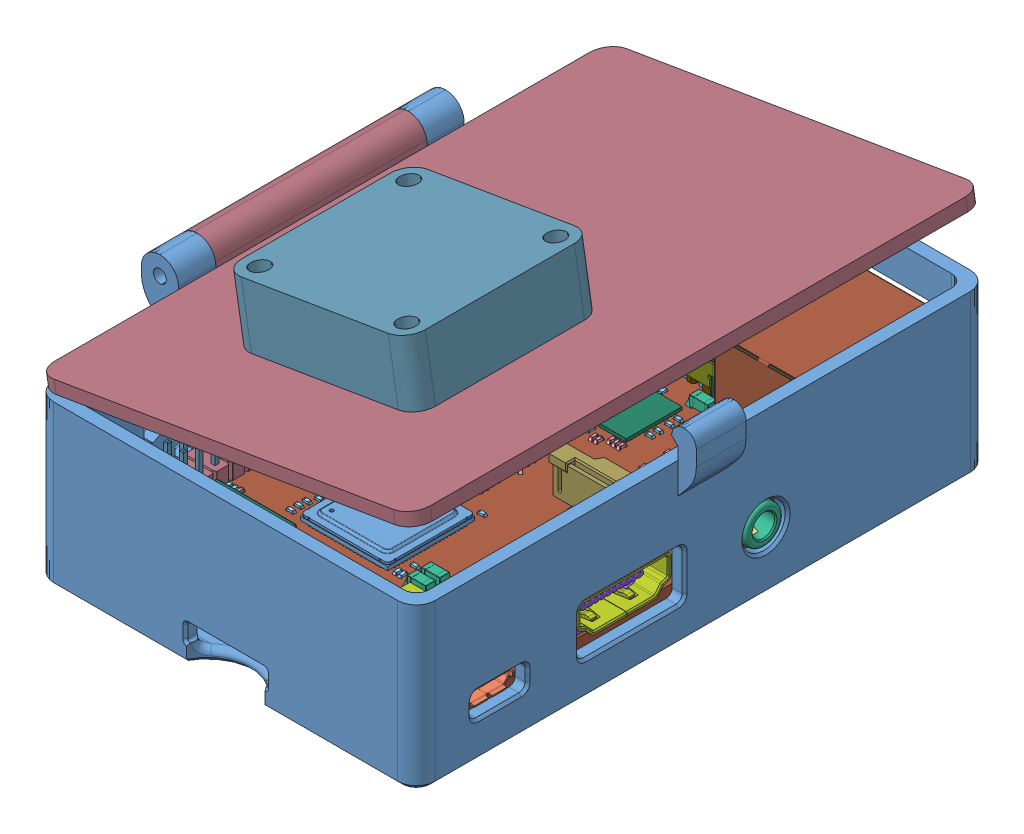
SolidWorks assembly 树莓派盒子组装, configuration 默认. Lengths in mm.
Overall size (70.85 46 92.2).
306 component instances, 68 part files, 8 mates.
Components (placement in the parent):
- 树莓派盒子-1: 树莓派盒子 [默认] at (-103.3103 -16.291 0) size (70.4 32 92.2)
- raspberry_pi_3_b_plus.stp-1: raspberry_pi_3_b_plus.stp [默认] at (-72.6103 -11.291 -45.2) x (0 0 -1) z (0 1 0) size (87.29 58.46 20.03)
  - micro_usb_connector v17.stp-1: micro_usb_connector v17.stp [默认] at (-31.9022 -25.6898 1.6) x (0 -1 0) z (0 0 1) size (5.84 7.77 3.4)
    - shield.stp-1: shield.stp [默认] at origin size (5.84 7.77 3.4)
    - socket_housing.stp-1: socket_housing.stp [默认] at origin size (4.25 6.85 2.15)
    - socket_plate.stp-1: socket_plate.stp [默认] at origin size (3.38 6.8 0.31)
    - terminal.stp-1: terminal.stp [默认] at origin size (3.22 0.35 1.72)
    - terminal.stp-2: terminal.stp [默认] at (0 -1.3 0) size (3.22 0.35 1.72)
    - terminal.stp-3: terminal.stp [默认] at (0 -0.65 0) size (3.22 0.35 1.72)
    - terminal.stp-4: terminal.stp [默认] at (0 0.65 0) size (3.22 0.35 1.72)
    - terminal.stp-5: terminal.stp [默认] at (0 1.3 0) size (3.22 0.35 1.72)
  - sd_card_slot_molex v11.stp-1: sd_card_slot_molex v11.stp [默认] at (-35.5259 0.0195 0) x (0 1 0) z (-1 0 0) size (12 1.5 11.41)
    - housing.stp-1: housing.stp [默认] at origin size (12 1.43 11.41)
      - shell.stp-1: shell.stp [默认] at origin size (12 1.43 11.41)
    - leads.stp-1: leads.stp [默认] at origin size (10.97 1.32 10.44)
      - Component12.stp-1: Component12.stp [默认] at origin size (0.75 1.14 7.86)
      - Component13.stp-1: Component13.stp [默认] at (-1.1 0 0) size (0.75 1.16 8.16)
      - Component14.stp-1: Component14.stp [默认] at (-3.3 0 0) size (0.75 1.13 7.81)
      - Component12.stp-2: Component12.stp [默认] at (-2.2 0 0) size (0.75 1.14 7.86)
      - Component12.stp-3: Component12.stp [默认] at (-4.4 0 0) size (0.75 1.14 7.86)
      - Component12.stp-4: Component12.stp [默认] at (-6.6 0 0) size (0.75 1.14 7.86)
      - Component12.stp-5: Component12.stp [默认] at (-7.7 0 0) size (0.75 1.14 7.86)
      - Component15.stp-1: Component15.stp [默认] at origin size (1.57 1.27 4.5)
      - Component16.stp-1: Component16.stp [默认] at origin size (1.37 1.25 4.89)
      - Component14.stp-2: Component14.stp [默认] at (-5.5 0 0) size (0.75 1.13 7.81)
    - base.stp-1: base.stp [默认] at origin size (11.85 1.42 10.4)
  - Pin Header 20x2 TH Pitch 2.54mm v1.stp-1: Pin Header 20x2 TH Pitch 2.54mm v1.stp [默认] at (-34.0983 24.2639 1.6) size (50.8 5.08 10)
    - spacers.stp-1: spacers.stp [默认] at origin size (50.8 5.08 2.54)
      - Component67.stp-1: Component67.stp [默认] at origin size (50.8 5.08 2.54)
    - pins.stp-1: pins.stp [默认] at origin size (48.9 3.17 10)
  - USB-A-stack-1x2.stp-1: USB-A-stack-1x2.stp [默认] at (35.9589 0.6157 1.6) size (17 15.83 20.03)
    - shell_1.stp-1: shell_1.stp [默认] at origin size (17 15.83 20.03)
      - outer.stp-1: outer.stp [默认] at origin size (17 15.83 20.03)
      - back_shell.stp-1: back_shell.stp [默认] at origin size (2.8 13.7 13.5)
      - mid_cover.stp-1: mid_cover.stp [默认] at origin size (8.5 12.4 5.09)
    - Component4.stp-1: Component4.stp [默认] at origin size (16.25 12.4 15.02)
      - Component5.stp-1: Component5.stp [默认] at origin size (16.25 12.4 15.02)
    - leads_1.stp-1: leads_1.stp [默认] at origin size (14.29 8.54 16.6)
      - top_lead.stp-1: top_lead.stp [默认] at origin size (14.29 1.54 16.6)
      - top_lead.stp-2: top_lead.stp [默认] at (0 -2.5 0) size (14.29 1.54 16.6)
      - top_lead.stp-3: top_lead.stp [默认] at (0 -7 0) size (14.29 1.54 16.6)
      - top_lead.stp-4: top_lead.stp [默认] at (0 -4.5 0) size (14.29 1.54 16.6)
      - bottom_lead.stp-1: bottom_lead.stp [默认] at origin size (11.67 1.54 7.97)
      - bottom_lead.stp-2: bottom_lead.stp [默认] at (0 -7 0) size (11.67 1.54 7.97)
      - bottom_lead.stp-3: bottom_lead.stp [默认] at (0 -2.5 0) size (11.67 1.54 7.97)
      - bottom_lead.stp-4: bottom_lead.stp [默认] at (0 -4.5 0) size (11.67 1.54 7.97)
  - USB-A-stack-1x2_1.stp-1: USB-A-stack-1x2_1.stp [默认] at (35.9589 19.0157 1.6) size (17 15.83 20.03)
    - shell_2.stp-1: shell_2.stp [默认] at origin size (17 15.83 20.03)
      - outer.stp-1: outer.stp [默认] at origin size (17 15.83 20.03)
      - back_shell.stp-1: back_shell.stp [默认] at origin size (2.8 13.7 13.5)
      - mid_cover.stp-1: mid_cover.stp [默认] at origin size (8.5 12.4 5.09)
    - Component4_1.stp-1: Component4_1.stp [默认] at origin size (16.25 12.4 15.02)
      - Component5.stp-1: Component5.stp [默认] at origin size (16.25 12.4 15.02)
    - leads_2.stp-1: leads_2.stp [默认] at origin size (14.29 8.54 16.6)
      - top_lead.stp-1: top_lead.stp [默认] at origin size (14.29 1.54 16.6)
      - top_lead.stp-2: top_lead.stp [默认] at (0 -2.5 0) size (14.29 1.54 16.6)
      - top_lead.stp-3: top_lead.stp [默认] at (0 -7 0) size (14.29 1.54 16.6)
      - top_lead.stp-4: top_lead.stp [默认] at (0 -4.5 0) size (14.29 1.54 16.6)
      - bottom_lead.stp-1: bottom_lead.stp [默认] at origin size (11.67 1.54 7.97)
      - bottom_lead.stp-2: bottom_lead.stp [默认] at (0 -7 0) size (11.67 1.54 7.97)
      - bottom_lead.stp-3: bottom_lead.stp [默认] at (0 -2.5 0) size (11.67 1.54 7.97)
      - bottom_lead.stp-4: bottom_lead.stp [默认] at (0 -4.5 0) size (11.67 1.54 7.97)
  - Pin Header 2x2 TH Pitch 2.54mm.stp-1: Pin Header 2x2 TH Pitch 2.54mm.stp [默认] at (17.7441 18.3632 1.6) size (5.08 5.08 10)
    - spacers_1.stp-1: spacers_1.stp [默认] at origin size (5.08 5.08 2.54)
      - Component5_1.stp-1: Component5_1.stp [默认] at origin size (5.08 5.08 2.54)
    - pins_1.stp-1: pins_1.stp [默认] at origin size (3.17 3.17 10)
  - EDAC_1743_RJ45_TH.stp-1: EDAC_1743_RJ45_TH.stp [默认] at (34.0212 -17.8853 1.5) x (0 1 0) z (0 0 1) size (16.2 21.37 16.96)
    - wiring.stp-1: wiring.stp [默认] at origin size (13.9 18.75 15.99)
      - rj45.stp-1: rj45.stp [默认] at origin size (13.46 13.45 4.49)
      - magnetics.stp-1: magnetics.stp [默认] at origin size (11.5 6.5 11.5)
      - leads_3.stp-1: leads_3.stp [默认] at origin size (13.9 7.95 8.72)
    - lights.stp-1: lights.stp [默认] at origin size (13.8 6.61 5.6)
      - led_org.stp-1: led_org.stp [默认] at (-5.37 0 2.2) size (3.04 5.2 4.86)
      - led_org.stp-2: led_org.stp [默认] at (5.37 0 2.2) size (3.04 5.2 4.86)
      - lights-0.stp-1: lights-0.stp [默认] at origin size (3.06 4.17 2.2)
      - lights-1.stp-1: lights-1.stp [默认] at origin size (3.06 4.17 2.2)
    - shell_3.stp-1: shell_3.stp [默认] at origin size (16.2 21.37 16.36)
    - base_1.stp-1: base_1.stp [默认] at origin size (15.6 20.75 16.5)
  - qfp16_3x2mm.stp-1: qfp16_3x2mm.stp [默认] at (-32.0595 4.9149 1.6) size (2.7 1.95 0.45)
    - Component1.stp-1: Component1.stp [默认] at origin size (2.5 1.75 0.4)
    - lead.stp-1: lead.stp [默认] at origin size (2.7 1.95 0.12)
  - wifi.stp-1: wifi.stp [默认] at origin size (10.5 13 2)
    - Component73.stp-1: Component73.stp [默认] at origin size (10.5 13 2)
  - crystal_dfn4.stp-1: crystal_dfn4.stp [默认] at (-16.2394 -5.9832 0) x (-1 0 0) z (0 0 -1) size (3.2 2.5 0.72)
    - Component2.stp-1: Component2.stp [默认] at origin size (3.2 2.5 0.3)
    - Component3.stp-1: Component3.stp [默认] at origin size (3.2 2.5 0.4)
    - Component4_2.stp-1: Component4_2.stp [默认] at origin size (2.9 2.3 0.2)
    - Component5_2.stp-1: Component5_2.stp [默认] at origin size (2.53 1.93 0.22)
  - crystal_dfn4.stp-2: crystal_dfn4.stp [默认] at (11.4677 1.4751 0) x (0 -1 0) z (0 0 -1) size (3.2 2.5 0.72)
    - Component2.stp-1: Component2.stp [默认] at origin size (3.2 2.5 0.3)
    - Component3.stp-1: Component3.stp [默认] at origin size (3.2 2.5 0.4)
    - Component4_2.stp-1: Component4_2.stp [默认] at origin size (2.9 2.3 0.2)
    - Component5_2.stp-1: Component5_2.stp [默认] at origin size (2.53 1.93 0.22)
  - pj-322.stp-1: pj-322.stp [默认] at (11.1035 -22.958 1.6) x (0 1 0) z (0 0 1) size (15 7.14 8.8)
    - tip_lead.stp-1: tip_lead.stp [默认] at origin size (9.11 7.14 8.34)
    - Component2_1.stp-1: Component2_1.stp [默认] at origin size (13.26 2.5 4.34)
    - Component3_1.stp-1: Component3_1.stp [默认] at origin size (11.45 1.41 8.71)
    - Component4_3.stp-1: Component4_3.stp [默认] at origin size (8.23 1.51 8.71)
    - pj-322-2.stp-1: pj-322-2.stp [默认] at origin size (15 7 7)
  - molex hdmi smt.stp-1: molex hdmi smt.stp [默认] at (-10.5578 -23.8041 1.6) size (15 12.18 8.27)
    - Component2_2.stp-1: Component2_2.stp [默认] at origin size (15 11.55 8.27)
    - molex hdmi smt-3.stp-1: molex hdmi smt-3.stp [默认] at origin size (14.9 10.35 6.23)
    - molex hdmi smt-4.stp-1: molex hdmi smt-4.stp [默认] at origin size (9.45 9.4 3.81)
    - molex hdmi smt-5.stp-1: molex hdmi smt-5.stp [默认] at origin size (8.45 9.4 3.11)
  - pcb.stp-1: pcb.stp [默认] at origin size (85 56 1.6)
  - te_1-1734248-5.stp-1: te_1-1734248-5.stp [默认] at (-38.8804 0.013 1.58) x (0 -1 0) z (-1 0 0) size (22.4 5.68 5.07)
  - te_1-1734248-5.stp-2: te_1-1734248-5.stp [默认] at (2.6829 -16.6511 1.58) x (0 1 0) z (1 0 0) size (22.4 5.68 5.07)
  - SOP-3_1.6mm.stp-1: SOP-3_1.6mm.stp [默认] at (-40.8905 -10.8155 0) x (-1 0 0) z (0 0 -1) size (1.6 1.56 0.65)
  - SOP-3_1.6mm.stp-2: SOP-3_1.6mm.stp [默认] at (-40.814 -18.4594 0) x (-1 0 0) z (0 0 -1) size (1.6 1.56 0.65)
  - SOP-3_1.6mm.stp-3: SOP-3_1.6mm.stp [默认] at (-16.6511 -13.2136 1.6) x (0 1 0) z (0 0 1) size (1.6 1.56 0.65)
  - SOP-3_1.6mm.stp-4: SOP-3_1.6mm.stp [默认] at (-16.6511 -11.1136 1.6) x (0 1 0) z (0 0 1) size (1.6 1.56 0.65)
  - qfn32_5mm.stp-1: qfn32_5mm.stp [默认] at (-29.2738 -12.9325 1.6) size (5.2 5.2 0.55)
  - qfn48_9mm.stp-1: qfn48_9mm.stp [默认] at (19.0565 -0.2385 1.6) size (9 9 0.6)
  - TSOP-6 2mm.stp-1: TSOP-6 2mm.stp [默认] at (14.2657 -10.6917 1.6) size (2 2.01 0.8)
  - TSOP-6 3mm.stp-1: TSOP-6 3mm.stp [默认] at (12.2743 17.7497 1.6) x (0 -1 0) z (0 0 1) size (3 2.91 0.8)
  - qfn80_12mm.stp-1: qfn80_12mm.stp [默认] at (0.9784 5.5219 0) x (-1 0 0) z (0 0 -1) size (12 12 0.6)
  - bcm2837.stp-1: bcm2837.stp [默认] at (-15.6667 3.4614 1.6) size (14 14 1.6)
  - wlbga140_5mm.stp-1: wlbga140_5mm.stp [默认] at (-30.4818 13.9472 1.6) size (4.47 5.27 0.51)
  - cap0603_03.stp-1: cap0603_03.stp [默认] at (6.2017 12.0599 1.6) size (2.34 0.91 0.83)
  - cap0603_03.stp-2: cap0603_03.stp [默认] at (-22.2778 -12.3124 1.6) size (2.34 0.91 0.83)
  - cap0603_03.stp-3: cap0603_03.stp [默认] at (-22.2778 -13.6124 1.6) size (2.34 0.91 0.83)
  - cap0603_03.stp-4: cap0603_03.stp [默认] at (-36.2901 -12.0302 1.6) size (2.34 0.91 0.83)
  - cap0603_03.stp-5: cap0603_03.stp [默认] at (-36.2901 -13.3302 1.6) size (2.34 0.91 0.83)
  - cap0603_03.stp-6: cap0603_03.stp [默认] at (-22.6025 -16.7071 1.6) x (0 -1 0) z (0 0 1) size (2.34 0.91 0.83)
  - cap0603_03.stp-7: cap0603_03.stp [默认] at (-31.9549 -9.0739 1.6) x (0 -1 0) z (0 0 1) size (2.34 0.91 0.83)
  - cap0603_03.stp-8: cap0603_03.stp [默认] at (-36.0614 -9.1191 1.6) x (0 -1 0) z (0 0 1) size (2.34 0.91 0.83)
  - cap0402.stp-1: cap0402.stp [默认] at (-1.6846 0.2009 1.6) size (1.37 0.6 0.51)
  - cap0402.stp-2: cap0402.stp [默认] at (-3.6165 0.1175 1.6) size (1.37 0.6 0.51)
  - cap0402.stp-3: cap0402.stp [默认] at (5.921 0.2585 1.6) size (1.37 0.6 0.51)
  - cap0402.stp-4: cap0402.stp [默认] at (3.9891 0.175 1.6) size (1.37 0.6 0.51)
  - cap0402.stp-5: cap0402.stp [默认] at (-2.0728 4.8443 1.6) size (1.37 0.6 0.51)
  - cap0402.stp-6: cap0402.stp [默认] at (-3.7336 5.7492 1.6) size (1.37 0.6 0.51)
  - cap0402.stp-7: cap0402.stp [默认] at (-1.7854 5.7598 1.6) size (1.37 0.6 0.51)
  - cap0402.stp-8: cap0402.stp [默认] at (1.0927 2.1177 1.6) size (1.37 0.6 0.51)
  - cap0402.stp-9: cap0402.stp [默认] at (-0.6601 2.5496 1.6) x (0 -1 0) z (0 0 1) size (1.37 0.6 0.51)
  - cap0402.stp-10: cap0402.stp [默认] at (-0.9045 7.6235 1.6) x (0 -1 0) z (0 0 1) size (1.37 0.6 0.51)
  - cap0402.stp-11: cap0402.stp [默认] at (4.5329 2.9706 1.6) size (1.37 0.6 0.51)
  - cap0402.stp-12: cap0402.stp [默认] at (6.3871 2.4516 1.6) x (0 -1 0) z (0 0 1) size (1.37 0.6 0.51)
  - cap0402.stp-13: cap0402.stp [默认] at (6.3503 5.2092 1.6) x (0 -1 0) z (0 0 1) size (1.37 0.6 0.51)
  - cap0402.stp-14: cap0402.stp [默认] at (4.9776 5.871 1.6) x (0 -1 0) z (0 0 1) size (1.37 0.6 0.51)
  - cap0402.stp-15: cap0402.stp [默认] at (2.183 -0.0836 1.6) x (0.707107 0.707107 0) z (0 0 1) size (1.37 0.6 0.51)
  - cap0402.stp-16: cap0402.stp [默认] at (2.5576 11.2194 1.6) x (0 -1 0) z (0 0 1) size (1.37 0.6 0.51)
  - cap0402.stp-17: cap0402.stp [默认] at (0.1286 11.1773 1.6) x (0 -1 0) z (0 0 1) size (1.37 0.6 0.51)
  - cap0402.stp-18: cap0402.stp [默认] at (2.2305 9.2075 1.6) size (1.37 0.6 0.51)
  - cap0402.stp-19: cap0402.stp [默认] at (5.9654 10.5975 1.6) size (1.37 0.6 0.51)
  - cap0402.stp-20: cap0402.stp [默认] at (6.7657 9.3479 1.6) size (1.37 0.6 0.51)
  - cap0402.stp-21: cap0402.stp [默认] at (-23.49 19.4613 1.6) size (1.37 0.6 0.51)
  - cap0402.stp-22: cap0402.stp [默认] at (-13.822 20.7849 1.6) size (1.37 0.6 0.51)
  - cap0402.stp-23: cap0402.stp [默认] at (-34.1053 3.5022 1.6) size (1.37 0.6 0.51)
  - cap0402.stp-24: cap0402.stp [默认] at (-31.4883 -16.4844 1.6) size (1.37 0.6 0.51)
  - cap0402.stp-25: cap0402.stp [默认] at (-30.9095 -8.8802 1.6) x (0 -1 0) z (0 0 1) size (1.37 0.6 0.51)
  - cap0402.stp-26: cap0402.stp [默认] at (-19.4165 -16.1422 1.6) x (0 -1 0) z (0 0 1) size (1.37 0.6 0.51)
  - cap0402.stp-27: cap0402.stp [默认] at (-36.281 -14.328 1.6) size (1.37 0.6 0.51)
  - cap0402.stp-28: cap0402.stp [默认] at (-19.435 -14.2136 1.6) x (0 -1 0) z (0 0 1) size (1.37 0.6 0.51)
  - cap0402.stp-29: cap0402.stp [默认] at (-22.334 -14.6736 1.6) size (1.37 0.6 0.51)
  - cap0402.stp-30: cap0402.stp [默认] at (21.8139 -19.5391 1.6) x (0 -1 0) z (0 0 1) size (1.37 0.6 0.51)
  - cap0402.stp-31: cap0402.stp [默认] at (14.9817 -13.1373 1.6) size (1.37 0.6 0.51)
  - cap0402.stp-32: cap0402.stp [默认] at (13.5717 -4.9875 1.6) size (1.37 0.6 0.51)
  - cap0402.stp-33: cap0402.stp [默认] at (13.5717 -4.1816 1.6) size (1.37 0.6 0.51)
  - cap0402.stp-34: cap0402.stp [默认] at (13.5938 -3.3757 1.6) size (1.37 0.6 0.51)
  - cap0402.stp-35: cap0402.stp [默认] at (12.6112 -2.2828 1.6) size (1.37 0.6 0.51)
  - cap0402.stp-36: cap0402.stp [默认] at (12.5671 -1.51 1.6) size (1.37 0.6 0.51)
  - cap0402.stp-37: cap0402.stp [默认] at (13.5496 0.709 1.6) size (1.37 0.6 0.51)
  - resistor_0402.stp-1: resistor_0402.stp [默认] at (13.5093 -0.0742 1.6) size (1.27 0.6 0.35)
  - resistor_0402.stp-2: resistor_0402.stp [默认] at (13.5249 2.0611 1.6) size (1.27 0.6 0.35)
  - resistor_0402.stp-3: resistor_0402.stp [默认] at (13.7425 5.6111 1.6) size (1.27 0.6 0.35)
  - resistor_0402.stp-4: resistor_0402.stp [默认] at (20.9328 7.1813 1.6) x (0 -1 0) z (0 0 1) size (1.27 0.6 0.35)
  - resistor_0402.stp-5: resistor_0402.stp [默认] at (21.7458 7.1931 1.6) x (0 -1 0) z (0 0 1) size (1.27 0.6 0.35)
  - cap0402.stp-38: cap0402.stp [默认] at (9.6972 18.2084 1.6) x (0 -1 0) z (0 0 1) size (1.37 0.6 0.51)
  - cap0402.stp-39: cap0402.stp [默认] at (14.7686 19.1245 1.6) x (0 -1 0) z (0 0 1) size (1.37 0.6 0.51)
  - resistor_0402.stp-6: resistor_0402.stp [默认] at (12.3038 -10.6968 1.6) size (1.27 0.6 0.35)
  - cap0402.stp-40: cap0402.stp [默认] at (12.2869 -9.7249 1.6) size (1.37 0.6 0.51)
  - cap0402.stp-41: cap0402.stp [默认] at (16.278 -9.6995 1.6) size (1.37 0.6 0.51)
  - resistor_0402.stp-7: resistor_0402.stp [默认] at (12.2911 -11.6977 1.6) size (1.27 0.6 0.35)
  - resistor_0402.stp-8: resistor_0402.stp [默认] at (16.2822 -10.7348 1.6) size (1.27 0.6 0.35)
  - resistor_0402.stp-9: resistor_0402.stp [默认] at (16.2949 -11.7484 1.6) size (1.27 0.6 0.35)
  - resistor_0402.stp-10: resistor_0402.stp [默认] at (12.2922 -13.2114 1.6) size (1.27 0.6 0.35)
  - resistor_0402.stp-11: resistor_0402.stp [默认] at (12.2703 -14.0987 1.6) size (1.27 0.6 0.35)
  - resistor_0402.stp-12: resistor_0402.stp [默认] at (6.2757 -16.9459 1.6) x (0 1 0) z (0 0 1) size (1.27 0.6 0.35)
  - resistor_0402.stp-13: resistor_0402.stp [默认] at (17.4427 -5.704 1.6) x (0 1 0) z (0 0 1) size (1.27 0.6 0.35)
  - resistor_0402.stp-14: resistor_0402.stp [默认] at (18.7432 -5.7156 1.6) x (0 1 0) z (0 0 1) size (1.27 0.6 0.35)
  - resistor_0402.stp-15: resistor_0402.stp [默认] at (20.5313 -5.7505 1.6) x (0 1 0) z (0 0 1) size (1.27 0.6 0.35)
  - resistor_0402.stp-16: resistor_0402.stp [默认] at (21.9594 -5.7389 1.6) x (0 1 0) z (0 0 1) size (1.27 0.6 0.35)
  - resistor_0402.stp-17: resistor_0402.stp [默认] at (24.5889 -0.5715 1.6) size (1.27 0.6 0.35)
  - resistor_0402.stp-18: resistor_0402.stp [默认] at (24.6319 0.218 1.6) size (1.27 0.6 0.35)
  - resistor_0402.stp-19: resistor_0402.stp [默认] at (14.7611 17.201 1.6) x (0 -1 0) z (0 0 1) size (1.27 0.6 0.35)
  - resistor_0402.stp-20: resistor_0402.stp [默认] at (4.9081 18.0957 1.6) x (0 -1 0) z (0 0 1) size (1.27 0.6 0.35)
  - resistor_0402.stp-21: resistor_0402.stp [默认] at (-7.0309 -3.1276 1.6) x (0 -1 0) z (0 0 1) size (1.27 0.6 0.35)
  - resistor_0402.stp-22: resistor_0402.stp [默认] at (-19.7233 -4.9873 1.6) x (0 -1 0) z (0 0 1) size (1.27 0.6 0.35)
  - resistor_0402.stp-23: resistor_0402.stp [默认] at (-21.9429 12.7546 1.6) x (0 -1 0) z (0 0 1) size (1.27 0.6 0.35)
  - resistor_0402.stp-24: resistor_0402.stp [默认] at (-20.6248 12.7941 1.6) x (0 -1 0) z (0 0 1) size (1.27 0.6 0.35)
  - resistor_0402.stp-25: resistor_0402.stp [默认] at (-19.3726 12.7414 1.6) x (0 -1 0) z (0 0 1) size (1.27 0.6 0.35)
  - resistor_0402.stp-26: resistor_0402.stp [默认] at (-18.1072 12.0428 1.6) x (0 -1 0) z (0 0 1) size (1.27 0.6 0.35)
  - resistor_0402.stp-27: resistor_0402.stp [默认] at (-11.6643 11.6022 1.6) size (1.27 0.6 0.35)
  - resistor_0402.stp-28: resistor_0402.stp [默认] at (-21.8944 -4.3988 1.6) size (1.27 0.6 0.35)
  - resistor_0402.stp-29: resistor_0402.stp [默认] at (-21.8845 -5.2127 1.6) size (1.27 0.6 0.35)
  - resistor_0402.stp-30: resistor_0402.stp [默认] at (-34.6286 7.0225 1.6) size (1.27 0.6 0.35)
  - resistor_0402.stp-31: resistor_0402.stp [默认] at (-34.6177 6.0172 1.6) size (1.27 0.6 0.35)
  - resistor_0402.stp-32: resistor_0402.stp [默认] at (-23.5017 21.2684 1.6) size (1.27 0.6 0.35)
  - resistor_0402.stp-33: resistor_0402.stp [默认] at (-23.4752 20.3668 1.6) size (1.27 0.6 0.35)
  - resistor_0402.stp-34: resistor_0402.stp [默认] at (-27.0587 -20.8199 1.6) size (1.27 0.6 0.35)
  - resistor_0402.stp-35: resistor_0402.stp [默认] at (-29.641 -17.6073 1.6) x (0 1 0) z (0 0 1) size (1.27 0.6 0.35)
  - resistor_0402.stp-36: resistor_0402.stp [默认] at (-28.8414 -17.6167 1.6) x (0 1 0) z (0 0 1) size (1.27 0.6 0.35)
  - resistor_0402.stp-37: resistor_0402.stp [默认] at (-19.1723 -12.1871 1.6) x (0 1 0) z (0 0 1) size (1.27 0.6 0.35)
  - resistor_0402.stp-38: resistor_0402.stp [默认] at (-18.3875 -11.105 1.6) x (0 1 0) z (0 0 1) size (1.27 0.6 0.35)
  - cap0402.stp-42: cap0402.stp [默认] at (-22.4123 -11.2455 1.6) size (1.37 0.6 0.51)
  - resistor_0402.stp-39: resistor_0402.stp [默认] at (-1.3556 -21.6749 1.6) size (1.27 0.6 0.35)
  - resistor_0402.stp-40: resistor_0402.stp [默认] at (-1.3556 -22.6419 1.6) size (1.27 0.6 0.35)
  - cap1206.stp-1: cap1206.stp [默认] at (7.9842 7.8874 1.6) size (4.14 2 1.61)
  - cap1206.stp-2: cap1206.stp [默认] at (-25.9964 -19.3212 1.6) size (4.14 2 1.61)
  - cap1206.stp-3: cap1206.stp [默认] at (-36.5363 -17.3583 1.6) x (0 1 0) z (0 0 1) size (4.14 2 1.61)
  - cap1206.stp-4: cap1206.stp [默认] at (-22.3159 -8.6166 1.6) x (0 1 0) z (0 0 1) size (4.14 2 1.61)
  - cap1206.stp-5: cap1206.stp [默认] at (-20.0447 -8.6166 1.6) x (0 1 0) z (0 0 1) size (4.14 2 1.61)
  - cap1206.stp-6: cap1206.stp [默认] at (-26.8904 -24.2006 1.6) x (0 1 0) z (0 0 1) size (4.14 2 1.61)
  - cap1206.stp-7: cap1206.stp [默认] at (23.3268 10.3578 1.6) x (0 1 0) z (0 0 1) size (4.14 2 1.61)
  - cap1206.stp-8: cap1206.stp [默认] at (23.886 19.0543 1.6) x (0 1 0) z (0 0 1) size (4.14 2 1.61)
  - cap1206.stp-9: cap1206.stp [默认] at (25.6036 -6.141 1.6) x (0 1 0) z (0 0 1) size (4.14 2 1.61)
  - cap1206.stp-10: cap1206.stp [默认] at (16.4512 -16.6927 1.6) x (0 1 0) z (0 0 1) size (4.14 2 1.61)
  - cap1206.stp-11: cap1206.stp [默认] at (17.7022 -20.3318 1.6) size (4.14 2 1.61)
  - cap0603_03.stp-9: cap0603_03.stp [默认] at (-16.8344 0.8188 -0.0007) x (-1 0 0) z (0 0 -1) size (2.34 0.91 0.83)
  - cap0603_03.stp-10: cap0603_03.stp [默认] at (-16.6946 6.8765 -0.0007) x (-1 0 0) z (0 0 -1) size (2.34 0.91 0.83)
  - cap0603_03.stp-11: cap0603_03.stp [默认] at (-40.1331 -7.592 -0.0007) x (-1 0 0) z (0 0 -1) size (2.34 0.91 0.83)
  - cap0603_03.stp-12: cap0603_03.stp [默认] at (13.801 -4.8435 -0.0007) x (-1 0 0) z (0 0 -1) size (2.34 0.91 0.83)
  - cap0603_03.stp-13: cap0603_03.stp [默认] at (22.8947 7.0224 -0.0007) x (-1 0 0) z (0 0 -1) size (2.34 0.91 0.83)
  - cap0603_03.stp-14: cap0603_03.stp [默认] at (21.8412 4.9066 -0.0007) x (0 1 0) z (0 0 -1) size (2.34 0.91 0.83)
  - cap0603_03.stp-15: cap0603_03.stp [默认] at (-11.6562 12.1885 -0.0007) x (0 1 0) z (0 0 -1) size (2.34 0.91 0.83)
  - resistor_0402.stp-41: resistor_0402.stp [默认] at (-40.4693 -16.2711 0) x (0 1 0) z (0 0 -1) size (1.27 0.6 0.35)
  - resistor_0402.stp-42: resistor_0402.stp [默认] at (-38.4065 -15.2729 0) x (0 1 0) z (0 0 -1) size (1.27 0.6 0.35)
  - resistor_0402.stp-43: resistor_0402.stp [默认] at (-40.3279 -13.3183 0) x (0 1 0) z (0 0 -1) size (1.27 0.6 0.35)
  - resistor_0402.stp-44: resistor_0402.stp [默认] at (-41.509 -13.3515 0) x (0 1 0) z (0 0 -1) size (1.27 0.6 0.35)
  - resistor_0402.stp-45: resistor_0402.stp [默认] at (-33.0196 -7.5021 0) x (0 1 0) z (0 0 -1) size (1.27 0.6 0.35)
  - resistor_0402.stp-46: resistor_0402.stp [默认] at (-26.8703 5.0577 0) x (-1 0 0) z (0 0 -1) size (1.27 0.6 0.35)
  - resistor_0402.stp-47: resistor_0402.stp [默认] at (-22.4565 -0.6922 0) x (-1 0 0) z (0 0 -1) size (1.27 0.6 0.35)
  - resistor_0402.stp-48: resistor_0402.stp [默认] at (-23.3861 9.2989 0) x (-0.707107 -0.707107 0) z (0 0 -1) size (1.27 0.6 0.35)
  - resistor_0402.stp-49: resistor_0402.stp [默认] at (-9.0472 -4.0009 0) x (-1 0 0) z (0 0 -1) size (1.27 0.6 0.35)
  - resistor_0402.stp-50: resistor_0402.stp [默认] at (1.7048 -1.558 0) x (-1 0 0) z (0 0 -1) size (1.27 0.6 0.35)
  - resistor_0402.stp-51: resistor_0402.stp [默认] at (7.8768 5.1135 0) x (0 -1 0) z (0 0 -1) size (1.27 0.6 0.35)
  - resistor_0402.stp-52: resistor_0402.stp [默认] at (16.9042 9.1312 0) x (0 -1 0) z (0 0 -1) size (1.27 0.6 0.35)
  - resistor_0402.stp-53: resistor_0402.stp [默认] at (17.8087 9.1423 0) x (0 -1 0) z (0 0 -1) size (1.27 0.6 0.35)
  - resistor_0402.stp-54: resistor_0402.stp [默认] at (20.8307 4.3775 0) x (0 -1 0) z (0 0 -1) size (1.27 0.6 0.35)
  - resistor_0402.stp-55: resistor_0402.stp [默认] at (18.8675 -5.4278 0) x (0 -1 0) z (0 0 -1) size (1.27 0.6 0.35)
  - resistor_0402.stp-56: resistor_0402.stp [默认] at (23.2421 -0.9015 0) x (-1 0 0) z (0 0 -1) size (1.27 0.6 0.35)
  - resistor_0402.stp-57: resistor_0402.stp [默认] at (23.2421 0.6867 0) x (-1 0 0) z (0 0 -1) size (1.27 0.6 0.35)
  - cap0402.stp-43: cap0402.stp [默认] at (-20.9328 -4.704 0) x (1 0 0) z (0 0 -1) size (1.37 0.6 0.51)
  - cap0402.stp-44: cap0402.stp [默认] at (-20.4676 -3.7177 0) x (1 0 0) z (0 0 -1) size (1.37 0.6 0.51)
  - cap0402.stp-45: cap0402.stp [默认] at (-20.1419 -2.7314 0) x (1 0 0) z (0 0 -1) size (1.37 0.6 0.51)
  - cap0402.stp-46: cap0402.stp [默认] at (-20.5327 -1.438 0) x (1 0 0) z (0 0 -1) size (1.37 0.6 0.51)
  - ind2520.stp-1: ind2520.stp [默认] at (-33.8028 -16.3221 1.6) x (0 1 0) z (0 0 1) size (2.5 2 1.53)
  - ind2520.stp-2: ind2520.stp [默认] at (-33.9058 -9.5866 1.6) x (0 1 0) z (0 0 1) size (2.5 2 1.53)
  - ind2520.stp-3: ind2520.stp [默认] at (-24.8087 -16.2044 1.6) x (0 1 0) z (0 0 1) size (2.5 2 1.53)
  - ind2520.stp-4: ind2520.stp [默认] at (-24.7831 -9.5014 1.6) x (0 1 0) z (0 0 1) size (2.5 2 1.53)
  - ledra_0603.stp-1: ledra_0603.stp [默认] at (-41.4207 -16.546 1.6) size (1.2 1.7 0.6)
  - ledra_0603.stp-2: ledra_0603.stp [默认] at (-41.4207 -20.2157 1.6) size (1.2 1.7 0.6)
  - SOP-3.stp-1: SOP-3.stp [默认] at (-17.0907 -15.6679 1.6) x (0 1 0) z (0 0 1) size (3 2.71 1.05)
  - SOP-3 2.5mm.stp-1: SOP-3 2.5mm.stp [默认] at (7.1392 -13.3247 1.6) size (2.6 2.21 0.65)
  - capar2_1013.stp-1: capar2_1013.stp [默认] at (-11.0324 -15.0395 1.6) x (0 1 0) z (0 0 1) size (1.47 1 0.66)
  - capar2_1013.stp-2: capar2_1013.stp [默认] at (-9.5324 -15.0395 1.6) x (0 1 0) z (0 0 1) size (1.47 1 0.66)
  - capar2_1013.stp-3: capar2_1013.stp [默认] at (-8.0324 -15.0395 1.6) x (0 1 0) z (0 0 1) size (1.47 1 0.66)
  - capar2_1013.stp-4: capar2_1013.stp [默认] at (-6.5324 -15.0395 1.6) x (0 1 0) z (0 0 1) size (1.47 1 0.66)
  - TSOP-2 4mm.stp-1: TSOP-2 4mm.stp [默认] at (-23.9074 -24.0113 1.6) size (3.5 5.91 2.05)
  - cap0402.stp-47: cap0402.stp [默认] at (-22.0963 -2.7373 0) x (1 0 0) z (0 0 -1) size (1.37 0.6 0.51)
  - cap0402.stp-48: cap0402.stp [默认] at (-19.3215 0.4779 0) x (1 0 0) z (0 0 -1) size (1.37 0.6 0.51)
  - cap0402.stp-49: cap0402.stp [默认] at (-15.3356 -0.1607 0) x (1 0 0) z (0 0 -1) size (1.37 0.6 0.51)
  - cap0402.stp-50: cap0402.stp [默认] at (-11.702 -0.7333 0) x (1 0 0) z (0 0 -1) size (1.37 0.6 0.51)
  - cap0402.stp-51: cap0402.stp [默认] at (-8.9713 -5.0055 0) x (1 0 0) z (0 0 -1) size (1.37 0.6 0.51)
  - cap0402.stp-52: cap0402.stp [默认] at (-15.5999 -3.3979 0) x (1 0 0) z (0 0 -1) size (1.37 0.6 0.51)
  - cap0402.stp-53: cap0402.stp [默认] at (-21.6338 1.8653 0) x (1 0 0) z (0 0 -1) size (1.37 0.6 0.51)
  - cap0402.stp-54: cap0402.stp [默认] at (-20.9732 3.1205 0) x (1 0 0) z (0 0 -1) size (1.37 0.6 0.51)
  - cap0402.stp-55: cap0402.stp [默认] at (-16.8111 2.548 0) x (1 0 0) z (0 0 -1) size (1.37 0.6 0.51)
  - cap0402.stp-56: cap0402.stp [默认] at (-12.9132 3.1866 0) x (1 0 0) z (0 0 -1) size (1.37 0.6 0.51)
  - cap0402.stp-57: cap0402.stp [默认] at (-20.5107 5.1465 0) x (1 0 0) z (0 0 -1) size (1.37 0.6 0.51)
  - cap0402.stp-58: cap0402.stp [默认] at (-18.6168 5.7411 0) x (1 0 0) z (0 0 -1) size (1.37 0.6 0.51)
  - cap0402.stp-59: cap0402.stp [默认] at (-12.1204 6.4018 0) x (1 0 0) z (0 0 -1) size (1.37 0.6 0.51)
  - cap0402.stp-60: cap0402.stp [默认] at (-20.4887 6.4678 0) x (1 0 0) z (0 0 -1) size (1.37 0.6 0.51)
  - cap0402.stp-61: cap0402.stp [默认] at (-18.1783 9.7527 0) x (1 0 0) z (0 0 -1) size (1.37 0.6 0.51)
  - cap0402.stp-62: cap0402.stp [默认] at (11.5736 3.8589 0) x (1 0 0) z (0 0 -1) size (1.37 0.6 0.51)
  - cap0402.stp-63: cap0402.stp [默认] at (-19.3344 8.2178 0) x (0.707107 -0.707107 0) z (0 0 -1) size (1.37 0.6 0.51)
  - cap0402.stp-64: cap0402.stp [默认] at (-6.2738 10.481 0) x (0.707107 -0.707107 0) z (0 0 -1) size (1.37 0.6 0.51)
  - cap0402.stp-65: cap0402.stp [默认] at (-17.4936 8.4844 0) x (0 -1 0) z (0 0 -1) size (1.37 0.6 0.51)
  - cap0402.stp-66: cap0402.stp [默认] at (-14.4924 9.289 0) x (0 -1 0) z (0 0 -1) size (1.37 0.6 0.51)
  - cap0402.stp-67: cap0402.stp [默认] at (-13.2739 7.7737 0) x (0 -1 0) z (0 0 -1) size (1.37 0.6 0.51)
  - cap0402.stp-68: cap0402.stp [默认] at (-12.604 9.6696 0) x (0 -1 0) z (0 0 -1) size (1.37 0.6 0.51)
  - cap0402.stp-69: cap0402.stp [默认] at (-13.236 4.9424 0) x (0 -1 0) z (0 0 -1) size (1.37 0.6 0.51)
  - cap0402.stp-70: cap0402.stp [默认] at (-18.4815 -0.9351 0) x (0 -1 0) z (0 0 -1) size (1.37 0.6 0.51)
  - cap0402.stp-71: cap0402.stp [默认] at (-14.5884 2.4903 0) x (0 -1 0) z (0 0 -1) size (1.37 0.6 0.51)
  - cap0402.stp-72: cap0402.stp [默认] at (-16.5097 -0.9351 0) x (0 -1 0) z (0 0 -1) size (1.37 0.6 0.51)
  - cap0402.stp-73: cap0402.stp [默认] at (-15.1951 -1.9084 0) x (0 -1 0) z (0 0 -1) size (1.37 0.6 0.51)
  - cap0402.stp-74: cap0402.stp [默认] at (-12.5787 -2.0474 0) x (0 -1 0) z (0 0 -1) size (1.37 0.6 0.51)
  - cap0402.stp-75: cap0402.stp [默认] at (-6.04 0.8805 0) x (-0.707107 -0.707107 0) z (0 0 -1) size (1.37 0.6 0.51)
  - cap0402.stp-76: cap0402.stp [默认] at (-18.4562 -3.3619 0) x (0 -1 0) z (0 0 -1) size (1.37 0.6 0.51)
  - cap0402.stp-77: cap0402.stp [默认] at (-19.5306 -5.6624 0) x (0 -1 0) z (0 0 -1) size (1.37 0.6 0.51)
  - cap0402.stp-78: cap0402.stp [默认] at (-18.6837 -5.7003 0) x (0 -1 0) z (0 0 -1) size (1.37 0.6 0.51)
  - cap0402.stp-79: cap0402.stp [默认] at (-13.8427 -6.3828 0) x (0 -1 0) z (0 0 -1) size (1.37 0.6 0.51)
  - cap0402.stp-80: cap0402.stp [默认] at (-26.961 -15.7507 0) x (0 -1 0) z (0 0 -1) size (1.37 0.6 0.51)
  - cap0402.stp-81: cap0402.stp [默认] at (16.475 4.4456 0) x (0 -1 0) z (0 0 -1) size (1.37 0.6 0.51)
  - cap0402.stp-82: cap0402.stp [默认] at (16.7816 1.9239 0) x (0 -1 0) z (0 0 -1) size (1.37 0.6 0.51)
  - cap0402.stp-83: cap0402.stp [默认] at (18.0539 1.8856 0) x (0 -1 0) z (0 0 -1) size (1.37 0.6 0.51)
  - cap0402.stp-84: cap0402.stp [默认] at (18.8714 1.8856 0) x (0 -1 0) z (0 0 -1) size (1.37 0.6 0.51)
  - cap0402.stp-85: cap0402.stp [默认] at (21.3016 1.0902 0) x (0 -1 0) z (0 0 -1) size (1.37 0.6 0.51)
  - cap0402.stp-86: cap0402.stp [默认] at (20.7714 -1.1412 0) x (0 -1 0) z (0 0 -1) size (1.37 0.6 0.51)
  - cap0402.stp-87: cap0402.stp [默认] at (15.6457 -5.4269 0) x (0 -1 0) z (0 0 -1) size (1.37 0.6 0.51)
  - cap0402.stp-88: cap0402.stp [默认] at (16.4457 -5.4269 0) x (0 -1 0) z (0 0 -1) size (1.37 0.6 0.51)
  - cap0402.stp-89: cap0402.stp [默认] at (17.2457 -5.4269 0) x (0 -1 0) z (0 0 -1) size (1.37 0.6 0.51)
  - cap0402.stp-90: cap0402.stp [默认] at (23.2344 -3.9236 0) x (1 0 0) z (0 0 -1) size (1.37 0.6 0.51)
- 树莓派盒子-盖子-1: 树莓派盒子-盖子 [默认] at (-42.3325 20.5852 0) x (0 0 -1) z (0.986263 0.165181 0) size (92.2 5.8 67.4)
- 3010风扇-1: 3010风扇 [Default] at (-88.4254 14.8933 -47) x (0.986263 0.165181 0) z (0 0 1) size (30 10 30)
Mates (geometry in assembly coordinates):
- 重合1: coincident anti-aligned: plane of 树莓派盒子-1 through (-97.1103 -11.291 -64.2) normal (0 1 0); plane of raspberry_pi_3_b_plus.stp-1/pcb.stp-1 through (-72.6103 -11.291 -45.2) normal (0 -1 0)
- 同心1: concentric aligned: circle of 树莓派盒子-1; cylinder of raspberry_pi_3_b_plus.stp-1/pcb.stp-1 through (-48.1103 -11.291 -6.2) axis (0 1 0) radius 1.375
- 同心2: concentric anti-aligned: cylinder of 树莓派盒子-1 through (-97.1103 -11.291 -6.2) axis (0 -1 0) radius 4; cylinder of raspberry_pi_3_b_plus.stp-1/pcb.stp-1 through (-97.1103 -11.291 -6.2) axis (0 1 0) radius 1.375
- 同心3: concentric aligned: circle of 树莓派盒子-1; circle of 树莓派盒子-盖子-1
- 重合6: coincident aligned: plane of 树莓派盒子-1 through (-103.3103 -14.291 -92.2) normal (0 0 -1); plane of 树莓派盒子-盖子-1 through (-45.6216 22.0621 -92.2) normal (0 0 -1)
- 同心4: concentric aligned: circle of 树莓派盒子-盖子-1; cylinder of 3010风扇-1 through (-85.4666 15.3888 -44) axis (-0.165181 0.986263 0) radius 1.5
- 同心5: concentric aligned: circle of 树莓派盒子-盖子-1; circle of 3010风扇-1
- 重合7: coincident anti-aligned: plane of 树莓派盒子-盖子-1 through (-100.2606 12.9111 -89.2) normal (-0.165181 0.986263 0); plane of 3010风扇-1 through (-88.4254 14.8933 -47) normal (0.165181 -0.986263 0)
